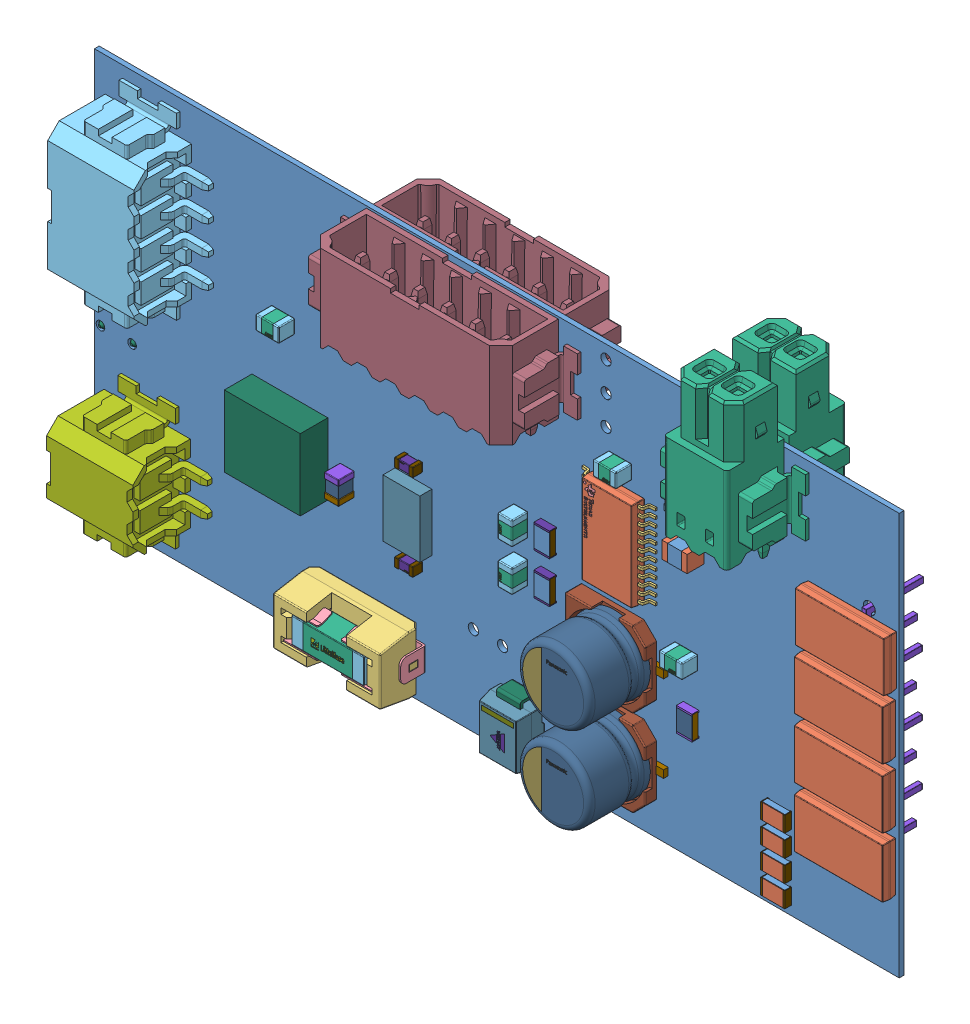
SolidWorks assembly placeholder, configuration Default. Lengths in mm.
Overall size (70.85 40.13 12.61).
391 component instances, 75 part files, 0 mates.
Components (placement in the parent):
- szpon.step-1: szpon.step [Default] at origin size (70.85 40.13 12.61)
  - Board.step-1: Board.step [Default] at origin size (70 35 0.41)
    - Open CASCADE STEP translator 7.5 1.1.1.step-1: Open CASCADE STEP translator 7.5 1.1.1.step [Default] at (0 0 -0.4115) size (70 35 0.41)
  - U2.step-1: U2.step [Default] at origin size (6.4 7.8 1.2)
    - IC_Texas_Instruments_DRV8873HPWPRQ1_eec.step-1: IC_Texas_Instruments_DRV8873HPWPRQ1_eec.step [Default] at (71.25 113.25 0) x (1 0 0) z (0 0 1) size (6.4 7.8 1.2)
      - body.step-1: body.step [Default] at origin size (4.4 7.8 1.15)
      - pins.step-1: pins.step [Default] at origin size (6.4 7.37 0.7)
      - logo.step-1: logo.step [Default] at (-2.2 0 1.2) size (1.02 4.27 0)
  - C20.step-1: C20.step [Default] at origin size (1.25 2.01 1.4)
    - Cap_AVX_08053C105KAT2A_eec.step-1: Cap_AVX_08053C105KAT2A_eec.step [Default] at (76.9 107.3 -0.4115) x (0 1 0) z (0 0 -1) size (2.01 1.25 1.4)
      - terminals.step-1: terminals.step [Default] at origin size (2.01 1.25 1.4)
      - body-0.step-1: body-0.step [Default] at origin size (1.01 1.25 1.4)
      - logo-1.step-1: logo-1.step [Default] at (0.096 0.222 1.4) size (0.7 0.24 0)
  - C17.step-1: C17.step [Default] at origin size (2.01 1.25 1.4)
    - Cap_AVX_08053C105KAT2A_eec.step-1: Cap_AVX_08053C105KAT2A_eec.step [Default] at (32.2 113.6 -0.4115) x (-1 0 0) z (0 0 -1) size (2.01 1.25 1.4)
      - terminals.step-1: terminals.step [Default] at origin size (2.01 1.25 1.4)
      - body-0.step-1: body-0.step [Default] at origin size (1.01 1.25 1.4)
      - logo-1.step-1: logo-1.step [Default] at (0.096 0.222 1.4) size (0.7 0.24 0)
  - C10.step-1: C10.step [Default] at origin size (2.01 1.25 1.4)
    - Cap_AVX_08053C105KAT2A_eec.step-1: Cap_AVX_08053C105KAT2A_eec.step [Default] at (77 107 0) size (2.01 1.25 1.4)
      - terminals.step-1: terminals.step [Default] at origin size (2.01 1.25 1.4)
      - body-0.step-1: body-0.step [Default] at origin size (1.01 1.25 1.4)
      - logo-1.step-1: logo-1.step [Default] at (0.096 0.222 1.4) size (0.7 0.24 0)
  - R3.step-1: R3.step [Default] at origin size (1.35 2.1 0.6)
    - 6522322464.step-1: 6522322464.step [Default] at (77.4 102.4 0) x (0 -1 0) z (0 0 1) size (2.1 1.35 0.6)
      - Terminal.step-1: Terminal.step [Default] at (-1.05 -0.675 0) size (0.15 1.35 0.6)
        - Open CASCADE STEP translator 6.8 3.2.1.step-1: Open CASCADE STEP translator 6.8 3.2.1.step [Default] at origin size (0.15 1.35 0.6)
      - Terminal.step-2: Terminal.step [Default] at (1.05 0.675 0) x (-1 0 0) z (0 0 1) size (0.15 1.35 0.6)
        - Open CASCADE STEP translator 6.8 3.2.1.step-1: Open CASCADE STEP translator 6.8 3.2.1.step [Default] at origin size (0.15 1.35 0.6)
      - Mid_Body.step-1: Mid_Body.step [Default] at (-1.05 -0.675 0) size (1.98 1.35 0.48)
      - Mark.step-1: Mark.step [Default] at (-0.9 -0.675 0.54) size (1.8 1.35 0.06)
  - R4.step-1: R4.step [Default] at origin size (0.8 1.6 0.95)
    - Res_Murata_NCP18WB473D03RB_eec.step-1: Res_Murata_NCP18WB473D03RB_eec.step [Default] at (77.4 102.4 -0.4115) x (0 1 0) z (0 0 -1) size (1.6 0.8 0.95)
      - 1.step-1: 1.step [Default] at origin size (1.6 0.8 0.95)
      - 2.step-1: 2.step [Default] at origin size (0.8 0.75 0.9)
      - Murata Logo 3.step-1: Murata Logo 3.step [Default] at (-0.5869 -1.4169 0.8251) size (0.36 0.08 0.1)
  - D1.step-1: D1.step [Default] at origin size (3.62 5.4 2.44)
    - Diode_Vishay_Semiconductor_Diodes_Division_SMBJ30A-E3-52_eec.step-1: Diode_Vishay_Semiconductor_Diodes_Division_SMBJ30A-E3-52_eec.step [Default] at (63 95.1 0) x (0 -1 0) z (0 0 1) size (5.4 3.62 2.44)
      - 1-2.step-1: 1-2.step [Default] at origin size (4.32 3.62 2.29)
      - 2-3.step-1: 2-3.step [Default] at origin size (5.4 2.08 1.5)
      - direction _Mark.step-1: direction _Mark.step [Default] at (6.1063 -3.5908 2.438) size (0.4 2.8 0)
      - Vishay.step-1: Vishay.step [Default] at (0.2194 -0.3703 2.4395) size (1.46 1.24 0)
  - R11.step-1: R11.step [Default] at origin size (2.1 1.35 0.6)
    - 6522337024.step-1: 6522337024.step [Default] at (85.1 99.2 0) x (1 0 0) z (0 0 1) size (2.1 1.35 0.6)
      - Terminal-1.step-1: Terminal-1.step [Default] at (-1.05 -0.675 0) size (0.15 1.35 0.6)
        - Open CASCADE STEP translator 6.8 3.2.1-4.step-1: Open CASCADE STEP translator 6.8 3.2.1-4.step [Default] at origin size (0.15 1.35 0.6)
      - Terminal-1.step-2: Terminal-1.step [Default] at (1.05 0.675 0) x (-1 0 0) z (0 0 1) size (0.15 1.35 0.6)
        - Open CASCADE STEP translator 6.8 3.2.1-4.step-1: Open CASCADE STEP translator 6.8 3.2.1-4.step [Default] at origin size (0.15 1.35 0.6)
      - Mid_Body-5.step-1: Mid_Body-5.step [Default] at (-1.05 -0.675 0) size (1.98 1.35 0.48)
      - Mark-6.step-1: Mark-6.step [Default] at (-0.9 -0.675 0.54) size (1.8 1.35 0.06)
  - R9.step-1: R9.step [Default] at origin size (2.1 1.35 0.6)
    - 6522337024.step-1: 6522337024.step [Default] at (85.1 95.4 0) x (1 0 0) z (0 0 1) size (2.1 1.35 0.6)
      - Terminal-1.step-1: Terminal-1.step [Default] at (-1.05 -0.675 0) size (0.15 1.35 0.6)
        - Open CASCADE STEP translator 6.8 3.2.1-4.step-1: Open CASCADE STEP translator 6.8 3.2.1-4.step [Default] at origin size (0.15 1.35 0.6)
      - Terminal-1.step-2: Terminal-1.step [Default] at (1.05 0.675 0) x (-1 0 0) z (0 0 1) size (0.15 1.35 0.6)
        - Open CASCADE STEP translator 6.8 3.2.1-4.step-1: Open CASCADE STEP translator 6.8 3.2.1-4.step [Default] at origin size (0.15 1.35 0.6)
      - Mid_Body-5.step-1: Mid_Body-5.step [Default] at (-1.05 -0.675 0) size (1.98 1.35 0.48)
      - Mark-6.step-1: Mark-6.step [Default] at (-0.9 -0.675 0.54) size (1.8 1.35 0.06)
  - R8.step-1: R8.step [Default] at origin size (2.1 1.35 0.6)
    - 6522337024.step-1: 6522337024.step [Default] at (85.1 93.5 0) x (1 0 0) z (0 0 1) size (2.1 1.35 0.6)
      - Terminal-1.step-1: Terminal-1.step [Default] at (-1.05 -0.675 0) size (0.15 1.35 0.6)
        - Open CASCADE STEP translator 6.8 3.2.1-4.step-1: Open CASCADE STEP translator 6.8 3.2.1-4.step [Default] at origin size (0.15 1.35 0.6)
      - Terminal-1.step-2: Terminal-1.step [Default] at (1.05 0.675 0) x (-1 0 0) z (0 0 1) size (0.15 1.35 0.6)
        - Open CASCADE STEP translator 6.8 3.2.1-4.step-1: Open CASCADE STEP translator 6.8 3.2.1-4.step [Default] at origin size (0.15 1.35 0.6)
      - Mid_Body-5.step-1: Mid_Body-5.step [Default] at (-1.05 -0.675 0) size (1.98 1.35 0.48)
      - Mark-6.step-1: Mark-6.step [Default] at (-0.9 -0.675 0.54) size (1.8 1.35 0.06)
  - F1.step-1: F1.step [Default] at origin size (9.73 5.03 3.81)
    - Fuse_Littelfuse_0154004_DR_eec.step-1: Fuse_Littelfuse_0154004_DR_eec.step [Default] at (49.5 95.5 0) x (1 0 0) z (0 0 1) size (9.73 5.03 3.81)
      - body-7.step-1: body-7.step [Default] at origin size (9.73 5.03 3.61)
      - terminals-8.step-1: terminals-8.step [Default] at origin size (9.73 3.4 3.61)
      - fuse terminals.step-1: fuse terminals.step [Default] at origin size (6.3 2.2 2.1)
      - fuse body.step-1: fuse body.step [Default] at origin size (4.3 2.2 2.1)
      - logo-9.step-1: logo-9.step [Default] at (0 -1.05 3.71) size (2.87 0.67 0)
  - D5.step-1: D5.step [Default] at origin size (3.2 3.2 10.6)
    - Diode_Vishay_TLLG4401_eec.step-1: Diode_Vishay_TLLG4401_eec.step [Default] at (92.9 117.3 0) x (0 1 0) z (0 0 1) size (3.2 3.2 10.6)
      - body.step-1: body.step [Default] at (0 0 1.4) size (3.2 3.2 4.7)
      - Leads.step-1: Leads.step [Default] at (0 0.175 1.4) x (1 0 0) z (0 -1 0) size (3.04 5.9 0.43)
  - D4.step-1: D4.step [Default] at origin size (3.2 3.2 10.6)
    - Diode_Vishay_TLLG4401_eec.step-1: Diode_Vishay_TLLG4401_eec.step [Default] at (92.8 112.1 0) x (0 1 0) z (0 0 1) size (3.2 3.2 10.6)
      - body.step-1: body.step [Default] at (0 0 1.4) size (3.2 3.2 4.7)
      - Leads.step-1: Leads.step [Default] at (0 0.175 1.4) x (1 0 0) z (0 -1 0) size (3.04 5.9 0.43)
  - D3.step-1: D3.step [Default] at origin size (3.2 3.2 10.6)
    - Diode_Vishay_TLLG4401_eec.step-1: Diode_Vishay_TLLG4401_eec.step [Default] at (92.8 106.9 0) x (0 1 0) z (0 0 1) size (3.2 3.2 10.6)
      - body.step-1: body.step [Default] at (0 0 1.4) size (3.2 3.2 4.7)
      - Leads.step-1: Leads.step [Default] at (0 0.175 1.4) x (1 0 0) z (0 -1 0) size (3.04 5.9 0.43)
  - D2.step-1: D2.step [Default] at origin size (3.2 3.2 10.6)
    - Diode_Vishay_TLLG4401_eec.step-1: Diode_Vishay_TLLG4401_eec.step [Default] at (92.8 101.7 0) x (0 1 0) z (0 0 1) size (3.2 3.2 10.6)
      - body.step-1: body.step [Default] at (0 0 1.4) size (3.2 3.2 4.7)
      - Leads.step-1: Leads.step [Default] at (0 0.175 1.4) x (1 0 0) z (0 -1 0) size (3.04 5.9 0.43)
  - C19.step-1: C19.step [Default] at origin size (1.25 2.01 1.4)
    - Cap_AVX_08053C105KAT2A_eec.step-1: Cap_AVX_08053C105KAT2A_eec.step [Default] at (62.6 106.4 0) x (0 -1 0) z (0 0 1) size (2.01 1.25 1.4)
      - terminals.step-1: terminals.step [Default] at origin size (2.01 1.25 1.4)
      - body-0.step-1: body-0.step [Default] at origin size (1.01 1.25 1.4)
      - logo-1.step-1: logo-1.step [Default] at (0.096 0.222 1.4) size (0.7 0.24 0)
  - C18.step-1: C18.step [Default] at origin size (2.01 1.25 1.4)
    - Cap_AVX_08053C105KAT2A_eec.step-1: Cap_AVX_08053C105KAT2A_eec.step [Default] at (88.2 110.9 -0.4115) x (1 0 0) z (0 0 -1) size (2.01 1.25 1.4)
      - terminals.step-1: terminals.step [Default] at origin size (2.01 1.25 1.4)
      - body-0.step-1: body-0.step [Default] at origin size (1.01 1.25 1.4)
      - logo-1.step-1: logo-1.step [Default] at (0.096 0.222 1.4) size (0.7 0.24 0)
  - C9.step-1: C9.step [Default] at origin size (1.25 2.01 1.4)
    - Cap_AVX_08053C105KAT2A_eec.step-1: Cap_AVX_08053C105KAT2A_eec.step [Default] at (62.6 110 0) x (0 -1 0) z (0 0 1) size (2.01 1.25 1.4)
      - terminals.step-1: terminals.step [Default] at origin size (2.01 1.25 1.4)
      - body-0.step-1: body-0.step [Default] at origin size (1.01 1.25 1.4)
      - logo-1.step-1: logo-1.step [Default] at (0.096 0.222 1.4) size (0.7 0.24 0)
  - C8.step-1: C8.step [Default] at origin size (1.25 2.01 1.4)
    - Cap_AVX_08053C105KAT2A_eec.step-1: Cap_AVX_08053C105KAT2A_eec.step [Default] at (79.25 118.25 0) x (0 1 0) z (0 0 1) size (2.01 1.25 1.4)
      - terminals.step-1: terminals.step [Default] at origin size (2.01 1.25 1.4)
      - body-0.step-1: body-0.step [Default] at origin size (1.01 1.25 1.4)
      - logo-1.step-1: logo-1.step [Default] at (0.096 0.222 1.4) size (0.7 0.24 0)
  - C4.step-1: C4.step [Default] at origin size (7.8 6.6 6.1)
    - Cap_Panasonic_EEEFT1V101AP_eec.step-1: Cap_Panasonic_EEEFT1V101AP_eec.step [Default] at (71.5 97.5 -0.4115) x (1 0 0) z (0 0 -1) size (7.8 6.6 6.1)
      - 1-10.step-1: 1-10.step [Default] at origin size (7.8 0.65 0.4)
      - 3.step-1: 3.step [Default] at origin size (6.3 6.3 5.6)
      - 4.step-1: 4.step [Default] at origin size (6.6 6.6 1.4)
      - 5.step-1: 5.step [Default] at origin size (3.85 4.89 0)
  - C3.step-1: C3.step [Default] at origin size (7.8 6.6 6.1)
    - Cap_Panasonic_EEEFT1V101AP_eec.step-1: Cap_Panasonic_EEEFT1V101AP_eec.step [Default] at (71.5 105 -0.4115) x (1 0 0) z (0 0 -1) size (7.8 6.6 6.1)
      - 1-10.step-1: 1-10.step [Default] at origin size (7.8 0.65 0.4)
      - 3.step-1: 3.step [Default] at origin size (6.3 6.3 5.6)
      - 4.step-1: 4.step [Default] at origin size (6.6 6.6 1.4)
      - 5.step-1: 5.step [Default] at origin size (3.85 4.89 0)
  - C2.step-1: C2.step [Default] at origin size (7.8 6.6 6.1)
    - Cap_Panasonic_EEEFT1V101AP_eec.step-1: Cap_Panasonic_EEEFT1V101AP_eec.step [Default] at (71.5 105 0) x (1 0 0) z (0 0 1) size (7.8 6.6 6.1)
      - 1-10.step-1: 1-10.step [Default] at origin size (7.8 0.65 0.4)
      - 3.step-1: 3.step [Default] at origin size (6.3 6.3 5.6)
      - 4.step-1: 4.step [Default] at origin size (6.6 6.6 1.4)
      - 5.step-1: 5.step [Default] at origin size (3.85 4.89 0)
  - C1.step-1: C1.step [Default] at origin size (7.8 6.6 6.1)
    - Cap_Panasonic_EEEFT1V101AP_eec.step-1: Cap_Panasonic_EEEFT1V101AP_eec.step [Default] at (71.5 97.5 0) x (1 0 0) z (0 0 1) size (7.8 6.6 6.1)
      - 1-10.step-1: 1-10.step [Default] at origin size (7.8 0.65 0.4)
      - 3.step-1: 3.step [Default] at origin size (6.3 6.3 5.6)
      - 4.step-1: 4.step [Default] at origin size (6.6 6.6 1.4)
      - 5.step-1: 5.step [Default] at origin size (3.85 4.89 0)
  - J3.step-1: J3.step [Default] at origin size (20.6 9.5 5)
    - 1814951.step-1: 1814951.step [Default] at (49.15 126.814 0) x (0 -1 0) z (-1 0 0) size (9.5 5 20.6)
      - ptsm_0.5-6-hho-2.5-smd-wh.step-1: ptsm_0.5-6-hho-2.5-smd-wh.step [Default] at (3.0388 17.2217 -6.15) size (9.5 5 20.6)
  - J2.step-1: J2.step [Default] at origin size (20.6 9.5 5)
    - 1814951.step-1: 1814951.step [Default] at (65.85 126.814 -0.4115) x (0 -1 0) z (1 0 0) size (9.5 5 20.6)
      - ptsm_0.5-6-hho-2.5-smd-wh.step-1: ptsm_0.5-6-hho-2.5-smd-wh.step [Default] at (3.0388 17.2217 -6.15) size (9.5 5 20.6)
  - X1.step-1: X1.step [Default] at origin size (3.2 5 1.05)
    - 6330668992.step-1: 6330668992.step [Default] at (53.25 106 0) size (3.2 5 1.05)
      - Extruded.step-1: Extruded.step [Default] at origin size (3.2 5 1.05)
  - U5.step-1: U5.step [Default] at origin size (6.6 6.2 2.4)
    - 6330566336.step-1: 6330566336.step [Default] at (42.5 106.25 0) size (6.6 6.2 2.4)
      - Extruded-11.step-1: Extruded-11.step [Default] at origin size (6.6 6.2 2.4)
  - U4.step-1: U4.step [Default] at origin size (4.9 6 1.76)
    - IC_Texas_Instruments_ISO7220ADR_eec.step-1: IC_Texas_Instruments_ISO7220ADR_eec.step [Default] at (32.3 118.5 -0.4115) x (0 1 0) z (0 0 -1) size (6 4.9 1.76)
      - IC_BODY.step-1: IC_BODY.step [Default] at (0 0 0.25) x (0 -1 0) z (0 0 1) size (4.9 3.9 1.5)
      - circle.step-1: circle.step [Default] at (-1.0726 1.9393 1.751) x (1 0 0) z (0 0 -1) size (0.4 0.4 0)
      - IC_LEG.step-1: IC_LEG.step [Default] at (-3 2.1095 0) x (1 0 0) z (0 -1 0) size (1.15 1.11 0.41)
      - IC_LEG.step-2: IC_LEG.step [Default] at (-3 0.8395 0) x (1 0 0) z (0 -1 0) size (1.15 1.11 0.41)
      - IC_LEG.step-3: IC_LEG.step [Default] at (-3 -0.4305 0) x (1 0 0) z (0 -1 0) size (1.15 1.11 0.41)
      - IC_LEG.step-4: IC_LEG.step [Default] at (-3 -1.7005 0) x (1 0 0) z (0 -1 0) size (1.15 1.11 0.41)
      - Texas Instruments.step-1: Texas Instruments.step [Default] at (0.0232 -1.7093 1.75) size (3.04 0.71 0.02)
      - IC_LEG_MIR8.step-1: IC_LEG_MIR8.step [Default] at (3 2.1095 0) x (-1 0 0) z (0 1 0) size (1.15 1.11 0.41)
      - IC_LEG_MIR8.step-2: IC_LEG_MIR8.step [Default] at (3 0.8395 0) x (-1 0 0) z (0 1 0) size (1.15 1.11 0.41)
      - IC_LEG_MIR8.step-3: IC_LEG_MIR8.step [Default] at (3 -0.4305 0) x (-1 0 0) z (0 1 0) size (1.15 1.11 0.41)
      - IC_LEG_MIR8.step-4: IC_LEG_MIR8.step [Default] at (3 -1.7005 0) x (-1 0 0) z (0 1 0) size (1.15 1.11 0.41)
  - U3.step-1: U3.step [Default] at origin size (7.8 6.4 1.2)
    - IC_Texas_Instruments_DRV8873HPWPRQ1_eec.step-1: IC_Texas_Instruments_DRV8873HPWPRQ1_eec.step [Default] at (82.75 102.75 -0.4115) x (0 1 0) z (0 0 -1) size (6.4 7.8 1.2)
      - body.step-1: body.step [Default] at origin size (4.4 7.8 1.15)
      - pins.step-1: pins.step [Default] at origin size (6.4 7.37 0.7)
      - logo.step-1: logo.step [Default] at (-2.2 0 1.2) size (1.02 4.27 0)
  - U1.step-1: U1.step [Default] at origin size (12 12 1.6)
    - 6522340704.step-1: 6522340704.step [Default] at (57 107.5 -0.4115) x (1 0 0) z (0 0 -1) size (12 12 1.6)
      - Body-12.step-1: Body-12.step [Default] at (-5 -5 0) size (10.01 10.01 1.55)
        - Open CASCADE STEP translator 6.8 5.2.1.step-1: Open CASCADE STEP translator 6.8 5.2.1.step [Default] at origin size (10.01 10.01 1.55)
      - Open CASCADE STEP translator 6.8 5.1.step-1: Open CASCADE STEP translator 6.8 5.1.step [Default] at (-5 -5 0.001) size (1.26 1.26 0.01)
      - Leader.step-1: Leader.step [Default] at (-5 -3.75 0) x (-1 0 0) z (0 0 1) size (1 0.22 0.88)
      - Leader.step-2: Leader.step [Default] at (-5 -3.25 0) x (-1 0 0) z (0 0 1) size (1 0.22 0.88)
      - Leader.step-3: Leader.step [Default] at (-5 -2.75 0) x (-1 0 0) z (0 0 1) size (1 0.22 0.88)
      - Leader.step-4: Leader.step [Default] at (-5 -2.25 0) x (-1 0 0) z (0 0 1) size (1 0.22 0.88)
      - Leader.step-5: Leader.step [Default] at (-5 -1.75 0) x (-1 0 0) z (0 0 1) size (1 0.22 0.88)
      - Leader.step-6: Leader.step [Default] at (-5 -1.25 0) x (-1 0 0) z (0 0 1) size (1 0.22 0.88)
      - Leader.step-7: Leader.step [Default] at (-5 -0.75 0) x (-1 0 0) z (0 0 1) size (1 0.22 0.88)
      - Leader.step-8: Leader.step [Default] at (-5 -0.25 0) x (-1 0 0) z (0 0 1) size (1 0.22 0.88)
      - Leader.step-9: Leader.step [Default] at (-5 0.25 0) x (-1 0 0) z (0 0 1) size (1 0.22 0.88)
      - Leader.step-10: Leader.step [Default] at (-5 0.75 0) x (-1 0 0) z (0 0 1) size (1 0.22 0.88)
      - Leader.step-11: Leader.step [Default] at (-5 1.25 0) x (-1 0 0) z (0 0 1) size (1 0.22 0.88)
      - Leader.step-12: Leader.step [Default] at (-5 1.75 0) x (-1 0 0) z (0 0 1) size (1 0.22 0.88)
      - Leader.step-13: Leader.step [Default] at (-5 2.25 0) x (-1 0 0) z (0 0 1) size (1 0.22 0.88)
      - Leader.step-14: Leader.step [Default] at (-5 2.75 0) x (-1 0 0) z (0 0 1) size (1 0.22 0.88)
      - Leader.step-15: Leader.step [Default] at (-5 3.25 0) x (-1 0 0) z (0 0 1) size (1 0.22 0.88)
      - Leader.step-16: Leader.step [Default] at (-5 3.75 0) x (-1 0 0) z (0 0 1) size (1 0.22 0.88)
      - Leader.step-17: Leader.step [Default] at (5 -3.75 0) size (1 0.22 0.88)
      - Leader.step-18: Leader.step [Default] at (5 -3.25 0) size (1 0.22 0.88)
      - Leader.step-19: Leader.step [Default] at (5 -2.75 0) size (1 0.22 0.88)
      - Leader.step-20: Leader.step [Default] at (5 -2.25 0) size (1 0.22 0.88)
      - Leader.step-21: Leader.step [Default] at (5 -1.75 0) size (1 0.22 0.88)
      - Leader.step-22: Leader.step [Default] at (5 -1.25 0) size (1 0.22 0.88)
      - Leader.step-23: Leader.step [Default] at (5 -0.75 0) size (1 0.22 0.88)
      - Leader.step-24: Leader.step [Default] at (5 -0.25 0) size (1 0.22 0.88)
      - Leader.step-25: Leader.step [Default] at (5 0.25 0) size (1 0.22 0.88)
      - Leader.step-26: Leader.step [Default] at (5 0.75 0) size (1 0.22 0.88)
      - Leader.step-27: Leader.step [Default] at (5 1.25 0) size (1 0.22 0.88)
      - Leader.step-28: Leader.step [Default] at (5 1.75 0) size (1 0.22 0.88)
      - Leader.step-29: Leader.step [Default] at (5 2.25 0) size (1 0.22 0.88)
      - Leader.step-30: Leader.step [Default] at (5 2.75 0) size (1 0.22 0.88)
      - Leader.step-31: Leader.step [Default] at (5 3.25 0) size (1 0.22 0.88)
      - Leader.step-32: Leader.step [Default] at (5 3.75 0) size (1 0.22 0.88)
      - Leader-13.step-1: Leader-13.step [Default] at (-3.75 -5 0) x (0 -1 0) z (0 0 1) size (1 0.22 0.88)
      - Leader-13.step-2: Leader-13.step [Default] at (-3.25 -5 0) x (0 -1 0) z (0 0 1) size (1 0.22 0.88)
      - Leader-13.step-3: Leader-13.step [Default] at (-2.75 -5 0) x (0 -1 0) z (0 0 1) size (1 0.22 0.88)
      - Leader-13.step-4: Leader-13.step [Default] at (-2.25 -5 0) x (0 -1 0) z (0 0 1) size (1 0.22 0.88)
      - Leader-13.step-5: Leader-13.step [Default] at (-1.75 -5 0) x (0 -1 0) z (0 0 1) size (1 0.22 0.88)
      - Leader-13.step-6: Leader-13.step [Default] at (-1.25 -5 0) x (0 -1 0) z (0 0 1) size (1 0.22 0.88)
      - Leader-13.step-7: Leader-13.step [Default] at (-0.75 -5 0) x (0 -1 0) z (0 0 1) size (1 0.22 0.88)
      - Leader-13.step-8: Leader-13.step [Default] at (-0.25 -5 0) x (0 -1 0) z (0 0 1) size (1 0.22 0.88)
      - Leader-13.step-9: Leader-13.step [Default] at (0.25 -5 0) x (0 -1 0) z (0 0 1) size (1 0.22 0.88)
      - Leader-13.step-10: Leader-13.step [Default] at (0.75 -5 0) x (0 -1 0) z (0 0 1) size (1 0.22 0.88)
      - Leader-13.step-11: Leader-13.step [Default] at (1.25 -5 0) x (0 -1 0) z (0 0 1) size (1 0.22 0.88)
      - Leader-13.step-12: Leader-13.step [Default] at (1.75 -5 0) x (0 -1 0) z (0 0 1) size (1 0.22 0.88)
      - Leader-13.step-13: Leader-13.step [Default] at (2.25 -5 0) x (0 -1 0) z (0 0 1) size (1 0.22 0.88)
      - Leader-13.step-14: Leader-13.step [Default] at (2.75 -5 0) x (0 -1 0) z (0 0 1) size (1 0.22 0.88)
      - Leader-13.step-15: Leader-13.step [Default] at (3.25 -5 0) x (0 -1 0) z (0 0 1) size (1 0.22 0.88)
      - Leader-13.step-16: Leader-13.step [Default] at (3.75 -5 0) x (0 -1 0) z (0 0 1) size (1 0.22 0.88)
      - Leader-13.step-17: Leader-13.step [Default] at (-3.75 5 0) x (0 1 0) z (0 0 1) size (1 0.22 0.88)
      - Leader-13.step-18: Leader-13.step [Default] at (-3.25 5 0) x (0 1 0) z (0 0 1) size (1 0.22 0.88)
      - Leader-13.step-19: Leader-13.step [Default] at (-2.75 5 0) x (0 1 0) z (0 0 1) size (1 0.22 0.88)
      - Leader-13.step-20: Leader-13.step [Default] at (-2.25 5 0) x (0 1 0) z (0 0 1) size (1 0.22 0.88)
      - Leader-13.step-21: Leader-13.step [Default] at (-1.75 5 0) x (0 1 0) z (0 0 1) size (1 0.22 0.88)
      - Leader-13.step-22: Leader-13.step [Default] at (-1.25 5 0) x (0 1 0) z (0 0 1) size (1 0.22 0.88)
      - Leader-13.step-23: Leader-13.step [Default] at (-0.75 5 0) x (0 1 0) z (0 0 1) size (1 0.22 0.88)
      - Leader-13.step-24: Leader-13.step [Default] at (-0.25 5 0) x (0 1 0) z (0 0 1) size (1 0.22 0.88)
      - Leader-13.step-25: Leader-13.step [Default] at (0.25 5 0) x (0 1 0) z (0 0 1) size (1 0.22 0.88)
      - Leader-13.step-26: Leader-13.step [Default] at (0.75 5 0) x (0 1 0) z (0 0 1) size (1 0.22 0.88)
      - Leader-13.step-27: Leader-13.step [Default] at (1.25 5 0) x (0 1 0) z (0 0 1) size (1 0.22 0.88)
      - Leader-13.step-28: Leader-13.step [Default] at (1.75 5 0) x (0 1 0) z (0 0 1) size (1 0.22 0.88)
      - Leader-13.step-29: Leader-13.step [Default] at (2.25 5 0) x (0 1 0) z (0 0 1) size (1 0.22 0.88)
      - Leader-13.step-30: Leader-13.step [Default] at (2.75 5 0) x (0 1 0) z (0 0 1) size (1 0.22 0.88)
      - Leader-13.step-31: Leader-13.step [Default] at (3.25 5 0) x (0 1 0) z (0 0 1) size (1 0.22 0.88)
      - Leader-13.step-32: Leader-13.step [Default] at (3.75 5 0) x (0 1 0) z (0 0 1) size (1 0.22 0.88)
  - SW1.step-1: SW1.step [Default] at origin size (4.5 5.5 2.47)
    - Switch_Panasonic_Electronic_Components_EVQ-PUD02K_eec.step-1: Switch_Panasonic_Electronic_Components_EVQ-PUD02K_eec.step [Default] at (26.9 106.4 -0.4115) x (0 1 0) z (0 0 -1) size (5.5 4.5 2.47)
      - 1-14.step-1: 1-14.step [Default] at (0 0.5 0.3) x (1 0 0) z (0 -1 0) size (5.5 2.47 4.5)
        - 1-15.step-1: 1-15.step [Default] at (0 -0.3 0) size (5.5 0.6 2.3)
        - 2-16.step-1: 2-16.step [Default] at origin size (0.19 0.51 0.8)
        - 3-17.step-1: 3-17.step [Default] at origin size (0.19 0.51 0.8)
        - 4-18.step-1: 4-18.step [Default] at origin size (2.4 0.05 0.56)
        - 5-19.step-1: 5-19.step [Default] at origin size (4.6 0.15 3.46)
        - 6.step-1: 6.step [Default] at origin size (1 0.44 0.73)
        - 7.step-1: 7.step [Default] at origin size (4.5 1 0.15)
        - 8.step-1: 8.step [Default] at origin size (4.5 1 0.12)
        - EVQPU-KB-02K.step-1: EVQPU-KB-02K.step [Default] at origin size (4.7 2.44 4.5)
        - Panasonic Logo.step-1: Panasonic Logo.step [Default] at (-4.236 1.5511 -1.5514) x (1 0 0) z (0 1 0) size (4.21 0.24 0.15)
  - R10.step-1: R10.step [Default] at origin size (2.1 1.35 0.6)
    - 6522337024.step-1: 6522337024.step [Default] at (85.1 97.3 0) x (1 0 0) z (0 0 1) size (2.1 1.35 0.6)
      - Terminal-1.step-1: Terminal-1.step [Default] at (-1.05 -0.675 0) size (0.15 1.35 0.6)
        - Open CASCADE STEP translator 6.8 3.2.1-4.step-1: Open CASCADE STEP translator 6.8 3.2.1-4.step [Default] at origin size (0.15 1.35 0.6)
      - Terminal-1.step-2: Terminal-1.step [Default] at (1.05 0.675 0) x (-1 0 0) z (0 0 1) size (0.15 1.35 0.6)
        - Open CASCADE STEP translator 6.8 3.2.1-4.step-1: Open CASCADE STEP translator 6.8 3.2.1-4.step [Default] at origin size (0.15 1.35 0.6)
      - Mid_Body-5.step-1: Mid_Body-5.step [Default] at (-1.05 -0.675 0) size (1.98 1.35 0.48)
      - Mark-6.step-1: Mark-6.step [Default] at (-0.9 -0.675 0.54) size (1.8 1.35 0.06)
  - R7.step-1: R7.step [Default] at origin size (1.35 2.1 0.6)
    - 6522330144.step-1: 6522330144.step [Default] at (65 106.4 0) x (0 1 0) z (0 0 1) size (2.1 1.35 0.6)
      - Terminal-2.step-1: Terminal-2.step [Default] at (-1.05 -0.675 0) size (0.15 1.35 0.6)
        - Open CASCADE STEP translator 6.8 3.2.1-20.step-1: Open CASCADE STEP translator 6.8 3.2.1-20.step [Default] at origin size (0.15 1.35 0.6)
      - Terminal-2.step-2: Terminal-2.step [Default] at (1.05 0.675 0) x (-1 0 0) z (0 0 1) size (0.15 1.35 0.6)
        - Open CASCADE STEP translator 6.8 3.2.1-20.step-1: Open CASCADE STEP translator 6.8 3.2.1-20.step [Default] at origin size (0.15 1.35 0.6)
      - Mid_Body-21.step-1: Mid_Body-21.step [Default] at (-1.05 -0.675 0) size (1.98 1.35 0.48)
      - Mark-22.step-1: Mark-22.step [Default] at (-0.9 -0.675 0.54) size (1.8 1.35 0.06)
  - R6.step-1: R6.step [Default] at origin size (2.1 1.35 0.6)
    - 6522331744.step-1: 6522331744.step [Default] at (54.6 98.8 -0.4115) x (1 0 0) z (0 0 -1) size (2.1 1.35 0.6)
      - Terminal-3.step-1: Terminal-3.step [Default] at (-1.05 -0.675 0) size (0.15 1.35 0.6)
        - Open CASCADE STEP translator 6.8 3.2.1-23.step-1: Open CASCADE STEP translator 6.8 3.2.1-23.step [Default] at origin size (0.15 1.35 0.6)
      - Terminal-3.step-2: Terminal-3.step [Default] at (1.05 0.675 0) x (-1 0 0) z (0 0 1) size (0.15 1.35 0.6)
        - Open CASCADE STEP translator 6.8 3.2.1-23.step-1: Open CASCADE STEP translator 6.8 3.2.1-23.step [Default] at origin size (0.15 1.35 0.6)
      - Mid_Body-24.step-1: Mid_Body-24.step [Default] at (-1.05 -0.675 0) size (1.98 1.35 0.48)
      - Mark-25.step-1: Mark-25.step [Default] at (-0.9 -0.675 0.54) size (1.8 1.35 0.06)
  - R5.step-1: R5.step [Default] at origin size (1.35 2.1 0.6)
    - 6522330144.step-1: 6522330144.step [Default] at (85.6 96.9 -0.4115) x (0 -1 0) z (0 0 -1) size (2.1 1.35 0.6)
      - Terminal-2.step-1: Terminal-2.step [Default] at (-1.05 -0.675 0) size (0.15 1.35 0.6)
        - Open CASCADE STEP translator 6.8 3.2.1-20.step-1: Open CASCADE STEP translator 6.8 3.2.1-20.step [Default] at origin size (0.15 1.35 0.6)
      - Terminal-2.step-2: Terminal-2.step [Default] at (1.05 0.675 0) x (-1 0 0) z (0 0 1) size (0.15 1.35 0.6)
        - Open CASCADE STEP translator 6.8 3.2.1-20.step-1: Open CASCADE STEP translator 6.8 3.2.1-20.step [Default] at origin size (0.15 1.35 0.6)
      - Mid_Body-21.step-1: Mid_Body-21.step [Default] at (-1.05 -0.675 0) size (1.98 1.35 0.48)
      - Mark-22.step-1: Mark-22.step [Default] at (-0.9 -0.675 0.54) size (1.8 1.35 0.06)
  - R2.step-1: R2.step [Default] at origin size (1.35 2.1 0.6)
    - 6522330144.step-1: 6522330144.step [Default] at (65 110 0) x (0 1 0) z (0 0 1) size (2.1 1.35 0.6)
      - Terminal-2.step-1: Terminal-2.step [Default] at (-1.05 -0.675 0) size (0.15 1.35 0.6)
        - Open CASCADE STEP translator 6.8 3.2.1-20.step-1: Open CASCADE STEP translator 6.8 3.2.1-20.step [Default] at origin size (0.15 1.35 0.6)
      - Terminal-2.step-2: Terminal-2.step [Default] at (1.05 0.675 0) x (-1 0 0) z (0 0 1) size (0.15 1.35 0.6)
        - Open CASCADE STEP translator 6.8 3.2.1-20.step-1: Open CASCADE STEP translator 6.8 3.2.1-20.step [Default] at origin size (0.15 1.35 0.6)
      - Mid_Body-21.step-1: Mid_Body-21.step [Default] at (-1.05 -0.675 0) size (1.98 1.35 0.48)
      - Mark-22.step-1: Mark-22.step [Default] at (-0.9 -0.675 0.54) size (1.8 1.35 0.06)
  - R1.step-1: R1.step [Default] at origin size (1.35 2.1 0.6)
    - 6522322464.step-1: 6522322464.step [Default] at (65.4 114.5 -0.4115) x (0 1 0) z (0 0 -1) size (2.1 1.35 0.6)
      - Terminal.step-1: Terminal.step [Default] at (-1.05 -0.675 0) size (0.15 1.35 0.6)
        - Open CASCADE STEP translator 6.8 3.2.1.step-1: Open CASCADE STEP translator 6.8 3.2.1.step [Default] at origin size (0.15 1.35 0.6)
      - Terminal.step-2: Terminal.step [Default] at (1.05 0.675 0) x (-1 0 0) z (0 0 1) size (0.15 1.35 0.6)
        - Open CASCADE STEP translator 6.8 3.2.1.step-1: Open CASCADE STEP translator 6.8 3.2.1.step [Default] at origin size (0.15 1.35 0.6)
      - Mid_Body.step-1: Mid_Body.step [Default] at (-1.05 -0.675 0) size (1.98 1.35 0.48)
      - Mark.step-1: Mark.step [Default] at (-0.9 -0.675 0.54) size (1.8 1.35 0.06)
  - J6.step-1: J6.step [Default] at origin size (9.5 15.6 5)
    - 1814935.step-1: 1814935.step [Default] at (26.436 112.35 0) x (1 0 0) z (0 -1 0) size (9.5 5 15.6)
      - ptsm_0.5-4-hho-2.5-smd-wh.step-1: ptsm_0.5-4-hho-2.5-smd-wh.step [Default] at (3.0388 17.2217 -6.15) size (9.5 5 15.6)
  - J5.step-1: J5.step [Default] at origin size (9.8 14 5)
    - 1815125.step-1: 1815125.step [Default] at (79.4 127.626 -0.4115) x (0 1 0) z (-1 0 0) size (14 5 9.8)
      - ptsm_0.5-2-hhi0_2.5-smd.step-1: ptsm_0.5-2-hhi0_2.5-smd.step [Default] at (3.0388 17.2217 -6.15) size (14 5 9.8)
  - J4.step-1: J4.step [Default] at origin size (9.8 14 5)
    - 1815125.step-1: 1815125.step [Default] at (86.1 127.626 0) x (0 1 0) z (1 0 0) size (14 5 9.8)
      - ptsm_0.5-2-hhi0_2.5-smd.step-1: ptsm_0.5-2-hhi0_2.5-smd.step [Default] at (3.0388 17.2217 -6.15) size (14 5 9.8)
  - J1.step-1: J1.step [Default] at origin size (9.5 10.6 5.7)
    - 1708004.step-1: 1708004.step [Default] at (26.335 101.766 0) x (0 -1 0) z (0 0 1) size (10.6 9.5 5.7)
      - PTSM_0.5_2_HH_2.5_SMD_WH_R32.step-1: PTSM_0.5_2_HH_2.5_SMD_WH_R32.step [Default] at (0.55 3.0388 17.2217) x (0 1 0) z (1 0 0) size (9.5 5.7 10.6)
  - C28.step-1: C28.step [Default] at origin size (1.25 2 1.4)
    - Cap_Kemet_C0805C106K8PACTU_eec.step-1: Cap_Kemet_C0805C106K8PACTU_eec.step [Default] at (47.5 105.5 0) x (0 1 0) z (0 0 1) size (0.5 1.25 1.4)
    - Cap_Kemet_C0805C106K8PACTU_eec-26.step-1: Cap_Kemet_C0805C106K8PACTU_eec-26.step [Default] at (47.5 105.5 0) x (0 1 0) z (0 0 1) size (0.5 1.25 1.4)
    - Cap_Kemet_C0805C106K8PACTU_eec-27.step-1: Cap_Kemet_C0805C106K8PACTU_eec-27.step [Default] at (47.5 105.5 0) x (0 1 0) z (0 0 1) size (1 1.15 1.3)
  - C27.step-1: C27.step [Default] at origin size (2.01 1.25 1.4)
    - Cap_AVX_08053C105KAT2A_eec.step-1: Cap_AVX_08053C105KAT2A_eec.step [Default] at (41.925 114.8 0) x (1 0 0) z (0 0 1) size (2.01 1.25 1.4)
      - terminals.step-1: terminals.step [Default] at origin size (2.01 1.25 1.4)
      - body-0.step-1: body-0.step [Default] at origin size (1.01 1.25 1.4)
      - logo-1.step-1: logo-1.step [Default] at (0.096 0.222 1.4) size (0.7 0.24 0)
  - C26.step-1: C26.step [Default] at origin size (1.45 2.2 1.45)
    - 6330677472.step-1: 6330677472.step [Default] at (47.6 110.6 -1.8615) size (1.45 1.2 1.45)
      - Extruded-28.step-1: Extruded-28.step [Default] at origin size (1.45 1.2 1.45)
    - 6330664832.step-1: 6330664832.step [Default] at (47.6 111.45 -1.8615) size (1.45 0.5 1.45)
      - Extruded-29.step-1: Extruded-29.step [Default] at origin size (1.45 0.5 1.45)
    - 6330664832.step-2: 6330664832.step [Default] at (47.6 109.75 -1.8615) size (1.45 0.5 1.45)
      - Extruded-29.step-1: Extruded-29.step [Default] at origin size (1.45 0.5 1.45)
  - C25.step-1: C25.step [Default] at origin size (2.01 1.25 1.4)
    - Cap_AVX_08053C105KAT2A_eec.step-1: Cap_AVX_08053C105KAT2A_eec.step [Default] at (62 115.5 -0.4115) x (1 0 0) z (0 0 -1) size (2.01 1.25 1.4)
      - terminals.step-1: terminals.step [Default] at origin size (2.01 1.25 1.4)
      - body-0.step-1: body-0.step [Default] at origin size (1.01 1.25 1.4)
      - logo-1.step-1: logo-1.step [Default] at (0.096 0.222 1.4) size (0.7 0.24 0)
  - C24.step-1: C24.step [Default] at origin size (2.01 1.25 1.4)
    - Cap_AVX_08053C105KAT2A_eec.step-1: Cap_AVX_08053C105KAT2A_eec.step [Default] at (52.9 115.3 -0.4115) x (-1 0 0) z (0 0 -1) size (2.01 1.25 1.4)
      - terminals.step-1: terminals.step [Default] at origin size (2.01 1.25 1.4)
      - body-0.step-1: body-0.step [Default] at origin size (1.01 1.25 1.4)
      - logo-1.step-1: logo-1.step [Default] at (0.096 0.222 1.4) size (0.7 0.24 0)
  - C23.step-1: C23.step [Default] at origin size (1.25 2.01 1.4)
    - Cap_AVX_08053C105KAT2A_eec.step-1: Cap_AVX_08053C105KAT2A_eec.step [Default] at (65 105 -0.4115) x (0 1 0) z (0 0 -1) size (2.01 1.25 1.4)
      - terminals.step-1: terminals.step [Default] at origin size (2.01 1.25 1.4)
      - body-0.step-1: body-0.step [Default] at origin size (1.01 1.25 1.4)
      - logo-1.step-1: logo-1.step [Default] at (0.096 0.222 1.4) size (0.7 0.24 0)
  - C22.step-1: C22.step [Default] at origin size (2.01 1.25 1.4)
    - Cap_AVX_08053C105KAT2A_eec.step-1: Cap_AVX_08053C105KAT2A_eec.step [Default] at (50.2 98.8 -0.4115) x (-1 0 0) z (0 0 -1) size (2.01 1.25 1.4)
      - terminals.step-1: terminals.step [Default] at origin size (2.01 1.25 1.4)
      - body-0.step-1: body-0.step [Default] at origin size (1.01 1.25 1.4)
      - logo-1.step-1: logo-1.step [Default] at (0.096 0.222 1.4) size (0.7 0.24 0)
  - C21.step-1: C21.step [Default] at origin size (1.25 2.01 1.4)
    - Cap_AVX_08053C105KAT2A_eec.step-1: Cap_AVX_08053C105KAT2A_eec.step [Default] at (47.5 102.1 -0.4115) x (0 -1 0) z (0 0 -1) size (2.01 1.25 1.4)
      - terminals.step-1: terminals.step [Default] at origin size (2.01 1.25 1.4)
      - body-0.step-1: body-0.step [Default] at origin size (1.01 1.25 1.4)
      - logo-1.step-1: logo-1.step [Default] at (0.096 0.222 1.4) size (0.7 0.24 0)
  - C16.step-1: C16.step [Default] at origin size (2.01 1.25 1.4)
    - Cap_AVX_08053C105KAT2A_eec.step-1: Cap_AVX_08053C105KAT2A_eec.step [Default] at (27.432 111.506 -0.4115) x (1 0 0) z (0 0 -1) size (2.01 1.25 1.4)
      - terminals.step-1: terminals.step [Default] at origin size (2.01 1.25 1.4)
      - body-0.step-1: body-0.step [Default] at origin size (1.01 1.25 1.4)
      - logo-1.step-1: logo-1.step [Default] at (0.096 0.222 1.4) size (0.7 0.24 0)
  - C15.step-1: C15.step [Default] at origin size (1.45 2.2 1.45)
    - 6330677472.step-1: 6330677472.step [Default] at (84.95 109.15 -1.8615) size (1.45 1.2 1.45)
      - Extruded-28.step-1: Extruded-28.step [Default] at origin size (1.45 1.2 1.45)
    - 6330664832.step-1: 6330664832.step [Default] at (84.95 108.3 -1.8615) size (1.45 0.5 1.45)
      - Extruded-29.step-1: Extruded-29.step [Default] at origin size (1.45 0.5 1.45)
    - 6330664832.step-2: 6330664832.step [Default] at (84.95 110 -1.8615) size (1.45 0.5 1.45)
      - Extruded-29.step-1: Extruded-29.step [Default] at origin size (1.45 0.5 1.45)
  - C14.step-1: C14.step [Default] at origin size (2 1.25 0.88)
    - Cap_KEMET_C0805C472J3HAC_eec.step-1: Cap_KEMET_C0805C472J3HAC_eec.step [Default] at (87.95 107.9 -0.4115) x (-1 0 0) z (0 0 -1) size (1 1.15 0.78)
    - Cap_KEMET_C0805C472J3HAC_eec-30.step-1: Cap_KEMET_C0805C472J3HAC_eec-30.step [Default] at (87.95 107.9 -0.4115) x (-1 0 0) z (0 0 -1) size (2 1.25 0.88)
    - Cap_KEMET_C0805C472J3HAC_eec-31.step-1: Cap_KEMET_C0805C472J3HAC_eec-31.step [Default] at (87.95 107.9 -0.4115) x (-1 0 0) z (0 0 -1) size (0.59 0.12 0)
  - C13.step-1: C13.step [Default] at origin size (1.25 2.01 1.4)
    - Cap_AVX_08053C105KAT2A_eec.step-1: Cap_AVX_08053C105KAT2A_eec.step [Default] at (88.25 102.75 -0.4115) x (0 1 0) z (0 0 -1) size (2.01 1.25 1.4)
      - terminals.step-1: terminals.step [Default] at origin size (2.01 1.25 1.4)
      - body-0.step-1: body-0.step [Default] at origin size (1.01 1.25 1.4)
      - logo-1.step-1: logo-1.step [Default] at (0.096 0.222 1.4) size (0.7 0.24 0)
  - C12.step-1: C12.step [Default] at origin size (1.6 0.8 0.87)
    - Cap_KEMET_C0603C272M5JACTU_eec.step-1: Cap_KEMET_C0603C272M5JACTU_eec.step [Default] at (53.25 102.25 0) x (-1 0 0) z (0 0 1) size (0.44 0.09 0)
    - Cap_KEMET_C0603C272M5JACTU_eec-32.step-1: Cap_KEMET_C0603C272M5JACTU_eec-32.step [Default] at (53.25 102.25 0) x (-1 0 0) z (0 0 1) size (0.9 0.72 0.77)
    - Cap_KEMET_C0603C272M5JACTU_eec-33.step-1: Cap_KEMET_C0603C272M5JACTU_eec-33.step [Default] at (53.25 102.25 0) x (-1 0 0) z (0 0 1) size (1.6 0.8 0.87)
  - C11.step-1: C11.step [Default] at origin size (1.6 0.8 0.87)
    - Cap_KEMET_C0603C272M5JACTU_eec.step-1: Cap_KEMET_C0603C272M5JACTU_eec.step [Default] at (53.25 109.75 0) size (0.44 0.09 0)
    - Cap_KEMET_C0603C272M5JACTU_eec-32.step-1: Cap_KEMET_C0603C272M5JACTU_eec-32.step [Default] at (53.25 109.75 0) size (0.9 0.72 0.77)
    - Cap_KEMET_C0603C272M5JACTU_eec-33.step-1: Cap_KEMET_C0603C272M5JACTU_eec-33.step [Default] at (53.25 109.75 0) size (1.6 0.8 0.87)
  - C7.step-1: C7.step [Default] at origin size (2.2 1.45 1.45)
    - 6330566576.step-1: 6330566576.step [Default] at (77.4 115.4 0) size (1.2 1.45 1.45)
      - Extruded-34.step-1: Extruded-34.step [Default] at origin size (1.2 1.45 1.45)
    - 6330566416.step-1: 6330566416.step [Default] at (76.55 115.4 0) size (0.5 1.45 1.45)
      - Extruded-35.step-1: Extruded-35.step [Default] at origin size (0.5 1.45 1.45)
    - 6330566416.step-2: 6330566416.step [Default] at (78.25 115.4 0) size (0.5 1.45 1.45)
      - Extruded-35.step-1: Extruded-35.step [Default] at origin size (0.5 1.45 1.45)
  - C6.step-1: C6.step [Default] at origin size (1.25 2 0.88)
    - Cap_KEMET_C0805C472J3HAC_eec.step-1: Cap_KEMET_C0805C472J3HAC_eec.step [Default] at (76.5 118.8492 0) x (0 -1 0) z (0 0 1) size (1 1.15 0.78)
    - Cap_KEMET_C0805C472J3HAC_eec-30.step-1: Cap_KEMET_C0805C472J3HAC_eec-30.step [Default] at (76.5 118.8492 0) x (0 -1 0) z (0 0 1) size (2 1.25 0.88)
    - Cap_KEMET_C0805C472J3HAC_eec-31.step-1: Cap_KEMET_C0805C472J3HAC_eec-31.step [Default] at (76.5 118.8492 0) x (0 -1 0) z (0 0 1) size (0.59 0.12 0)
  - C5.step-1: C5.step [Default] at origin size (2.01 1.25 1.4)
    - Cap_AVX_08053C105KAT2A_eec.step-1: Cap_AVX_08053C105KAT2A_eec.step [Default] at (71.25 118.5 0) x (1 0 0) z (0 0 1) size (2.01 1.25 1.4)
      - terminals.step-1: terminals.step [Default] at origin size (2.01 1.25 1.4)
      - body-0.step-1: body-0.step [Default] at origin size (1.01 1.25 1.4)
      - logo-1.step-1: logo-1.step [Default] at (0.096 0.222 1.4) size (0.7 0.24 0)
